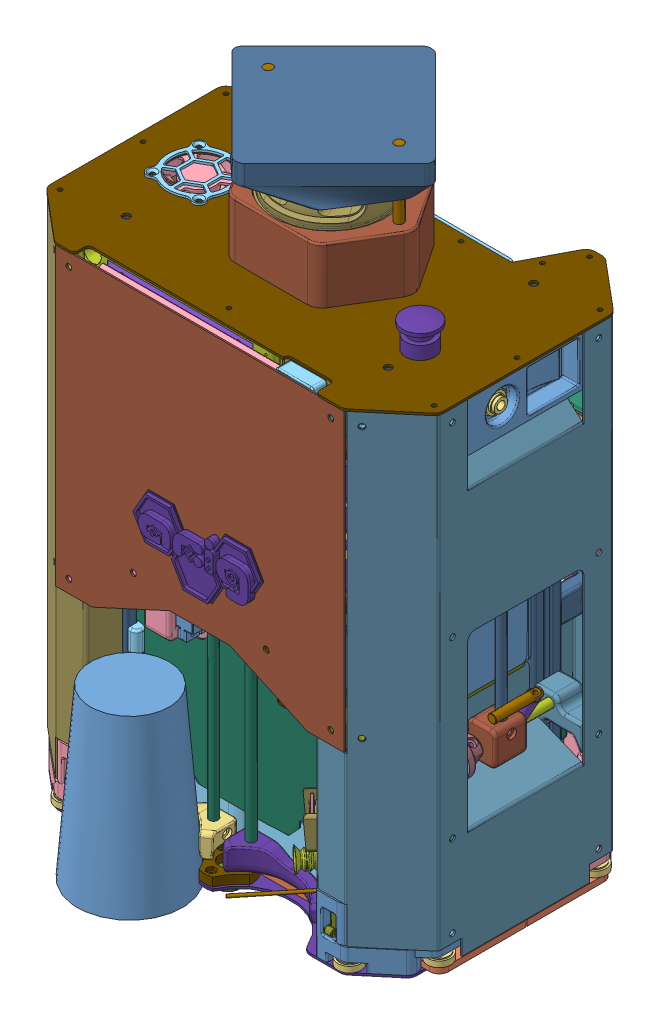
SolidWorks assembly _2021_RobotSecondaire_V1, configuration Default. Lengths in mm. (continued)
Components (placement in the parent): (continued)
- _Symétrie_Angle-4: _Symétrie_Angle [Défaut] at (-3.845 0 0) x (-1 0 0) z (0 0 -1) size (53.5 52 51.1)
  - _Symétrie_microswitchGaletAss-1: _Symétrie_microswitchGaletAss [Défaut] at (85.155 44 -75) x (0 -1 0) z (1 0 0) size (21.06 21.1 7)
    - _Symétrie_microswitchGalet02-1: _Symétrie_microswitchGalet02 [Défaut] at origin size (20 15 7)
    - _Symétrie_microswitchGalet01-1: _Symétrie_microswitchGalet01 [Défaut] at (1.7099 12.1145 0) x (0.996636 -0.081957 0) z (0 0 1) size (19 9 6)
  - _Symétrie_Angle_support-1: _Symétrie_Angle_support [Défaut] at (86.155 7 -50) size (53.5 52 49)
- PlaqueAvant-2: PlaqueAvant [Défaut] at (0 5.5 -40) x (-1 0 0) z (0 0 -1) size (250 17.2 51.5)
  - BillePorteuse2019-1: BillePorteuse2019 [Défaut] at (0 -6.2 30) size (16 10 16)
  - PlaqueAvant_Tole-1: PlaqueAvant_Tole [Défaut] at origin size (250 1.5 50)
  - PlaqueAvant_SupportBille-1: PlaqueAvant_SupportBille [Défaut] at (0 2.5 30) size (32 10 25.6)
  - RoulementAngle-1: RoulementAngle [Défaut] at (-96.8842 4.25 43.5) size (16 9.5 16)
  - RoulementAngle-2: RoulementAngle [Défaut] at (96.8842 4.25 43.5) size (16 9.5 16)
- _Symétrie_BrasLateral-2: _Symétrie_BrasLateral [Défaut] at (82 117.5 38.35) size (52.5 125.87 147.5)
  - _Symétrie_Access_HS-645_Rond-1: _Symétrie_Access_HS-645_Rond [Défaut] at (28 -10.2 -7.8) x (-0.986286 0.165048 0) z (-0.165048 -0.986286 0) size (24 5 24)
  - _Symétrie_Servo_HS-485-HB-1: _Symétrie_Servo_HS-485-HB [Default] at (28 -10.2 31.94) x (-1 0 0) z (0 0 1) size (19.81 54.15 42.74)
  - _Symétrie_Bras_AxePivot-1: _Symétrie_Bras_AxePivot [Default] at (28 -10.2 -16.3) x (0.492424 0.870356 0) z (0 0 1) size (6 6 80)
  - _Symétrie_Bras_Alu_TubeCarre_07.5-1: _Symétrie_Bras_Alu_TubeCarre_07.5 [Default] at (34.6477 1.5498 -55.3) x (0.870356 -0.492424 0) z (0.492424 0.870356 0) size (8 8 26)
  - _Symétrie_Bras_AxeButee-1: _Symétrie_Bras_AxeButee [Default] at (41.2954 13.2996 -59.3) x (0.492424 0.870356 0) z (0 0 -1) size (6 6 33)
  - _Symétrie_Bras_Rouleau-1: _Symétrie_Bras_Rouleau [Défaut] at (35.2953 -10.2 -38.75) x (0 0 -1) z (0 -1 0) size (24.5 22.96 102.46)
    - _Symétrie_Bras_Axe-1: _Symétrie_Bras_Axe [Default] at origin size (6 6 94)
    - _Symétrie_Bras_Pivot-1: _Symétrie_Bras_Pivot [Default] at (0 0 8) x (0 1 0) z (-1 0 0) size (22.5 23 22.5)
    - _Symétrie_Igus_Bague_d06-1: _Symétrie_Igus_Bague_d06 [Défaut] at (-12.25 -7.2953 0) size (10 12 12)
    - _Symétrie_Igus_Bague_d06-2: _Symétrie_Igus_Bague_d06 [Défaut] at (12.25 -7.2953 0) x (-1 0 0) z (0 0.759835 -0.650115) size (10 12 12)
  - _Symétrie_Bras_FixAxePivot-1: _Symétrie_Bras_FixAxePivot [Défaut] at (28 -10.2 -12.3) x (-0.870356 0.492424 0) z (-0.492424 -0.870356 0) size (24 14 24)
  - _Symétrie_Bras_SupportAxe-1: _Symétrie_Bras_SupportAxe [Défaut] at (18 -21.2 -88.35) x (0 0 -1) z (-1 0 0) size (18 26 35)
  - _Symétrie_Bras_SupportServo_Bottom-1: _Symétrie_Bras_SupportServo_Bottom [Défaut] at (8 -42.065 11.65) x (0 0 1) z (-1 0 0) size (18 22 35)
  - _Symétrie_Bras_SupportServo_Top-1: _Symétrie_Bras_SupportServo_Top [Défaut] at (8 19.815 11.65) x (-1 0 0) z (0 0 -1) size (39 18 44.5)
- LogoARIG2-1: LogoARIG2 [Défaut] at (-42.5 182 89.5) size (88.08 45.8 6.03)
- LogoARIG2-3: LogoARIG2 [Défaut] at (42.5 182 -89.5) x (-1 0 0) z (0 0 -1) size (88.08 45.8 6.03)
- Pneumatique2-2: Pneumatique2 [Défaut] at (-80 92 0) x (0 0 -1) z (1 0 0) size (118 63.5 92.8)
  - Pneumatique_Support2-1: Pneumatique_Support2 [Défaut] at (0 0 -10) size (118 15 27.1)
  - CroixPiquageRapideD06-1: CroixPiquageRapideD06 [Default] at (12.5 14.5 29.25) x (-1 0 0) z (0 -1 0) size (38 38 13)
  - CroixPiquageRapideD06-2: CroixPiquageRapideD06 [Default] at (-12.5 -6.5 29.25) x (1 0 0) z (0 1 0) size (38 38 13)
  - CapteurVide_CKD_PPE-V01A-H6-B-1: CapteurVide_CKD_PPE-V01A-H6-B [Défaut] at (12.5 14.5 52.75) x (0 -1 0) z (-1 0 0) size (37 43 15)
  - CapteurVide_CKD_PPE-V01A-H6-B-2: CapteurVide_CKD_PPE-V01A-H6-B [Défaut] at (-12.5 -6.5 52.75) x (0 1 0) z (1 0 0) size (37 43 15)
  - Electrovanne_CylindriqueD24_NC_12V-1: Electrovanne_CylindriqueD24_NC_12V [Default] at (12.5 -18.5 -2) x (0 0 1) z (-1 0 0) size (38.24 53 24.48)
  - Electrovanne_CylindriqueD24_NC_12V-2: Electrovanne_CylindriqueD24_NC_12V [Default] at (-12.5 26.5 -2) x (0 0 1) z (1 0 0) size (38.24 53 24.48)
  - Pneumatique_Fix-1: Pneumatique_Fix [Défaut] at (0 0 -2) x (-1 0 0) z (0 0 -1) size (75 8 14.55)
  - Pièce4^Pneumatique2-1: Pièce4^Pneumatique2 [Défaut] at (-9 -6.5 29.25) x (0 -1 0) z (1 0 0) size (24.78 14.3 44.64) (virtual)
  - Pièce5^Pneumatique2-1: Pièce5^Pneumatique2 [Défaut] at (16 14.5 29.25) x (0 -1 0) z (1 0 0) size (50.6 27.61 36.51) (virtual)
  - Pièce6^Pneumatique2-1: Pièce6^Pneumatique2 [Défaut] at (-16 -6.5 29.25) x (0 1 0) z (-1 0 0) size (29.52 27.83 36.35) (virtual)
  - Pièce7^Pneumatique2-1: Pièce7^Pneumatique2 [Défaut] at (9 14.5 29.25) x (0 1 0) z (-1 0 0) size (45.5 14.26 63.44) (virtual)
Mates (geometry in assembly coordinates):
- Coïncidente1: coincident: plane of assembly through (0 0 0) normal (0 1 0); plane of 2020_ADJ_Bouee-1 through (37.5 0 100) normal (0 1 0); plane of assembly
- Coïncidente2: coincident: plane of assembly through (0 0 0) normal (0 1 0); plane of 2020_ADJ_Bouee-2 through (-37.5 0 100) normal (0 1 0); plane of assembly
- Coïncidente3: coincident: plane of assembly through (0 0 0) normal (0 1 0); plane of 2020_ADJ_Bouee-3 through (37.5 0 -100) normal (0 1 0); plane of assembly
- Coïncidente4: coincident: plane of assembly through (0 0 0) normal (0 1 0); plane of 2020_ADJ_Bouee-4 through (-37.5 0 -100) normal (0 1 0); plane of assembly
- Coïncidente5: coincident: plane of assembly; plane of assembly; plane of 2020_ADJ_Bouee-1 through (37.5 0 100) normal (0 0 1); plane of 2020_ADJ_Bouee-2 through (-37.5 0 100) normal (0 0 1)
- Coïncidente6: coincident: plane of assembly; plane of assembly; plane of 2020_ADJ_Bouee-3 through (37.5 0 -100) normal (0 0 1); plane of 2020_ADJ_Bouee-4 through (-37.5 0 -100) normal (0 0 1)
- Coïncidente7: coincident: plane of assembly; plane of assembly; plane of 2020_ADJ_Bouee-1 through (37.5 0 100) normal (1 0 0); plane of 2020_ADJ_Bouee-3 through (37.5 0 -100) normal (1 0 0)
- Coïncidente8: coincident: plane of assembly; plane of assembly; plane of 2020_ADJ_Bouee-2 through (-37.5 0 100) normal (1 0 0); plane of 2020_ADJ_Bouee-4 through (-37.5 0 -100) normal (1 0 0)
- Symétrique1: symmetric: plane of assembly; plane of assembly; plane of 2020_ADJ_Bouee-1 through (37.5 0 100) normal (1 0 0); plane of 2020_ADJ_Bouee-2 through (-37.5 0 100) normal (1 0 0); plane of assembly
- Symétrique2: symmetric: plane of assembly; plane of assembly; plane of 2020_ADJ_Bouee-1 through (37.5 0 100) normal (0 0 1); plane of 2020_ADJ_Bouee-3 through (37.5 0 -100) normal (0 0 1); plane of assembly
- Distance1: distance = 100 mm: plane of assembly through (0 0 0) normal (0 0 1); plane of 2020_ADJ_Bouee-1 through (37.5 0 100) normal (0 0 1); plane of assembly
- Distance2: distance = 37.5 mm: plane of assembly through (0 0 0) normal (1 0 0); plane of 2020_ADJ_Bouee-1 through (37.5 0 100) normal (1 0 0); plane of assembly
- Coïncidente73: coincident: plane of VolumeRobot-1 through (0 0 0) normal (0 0 1); plane of assembly through (0 0 0) normal (0 0 1)
- Coïncidente74: coincident: plane of VolumeRobot-1 through (0 0 0) normal (0 1 0); plane of assembly through (0 0 0) normal (0 1 0)
- Coïncidente75: coincident: plane of VolumeRobot-1 through (0 0 0) normal (1 0 0); plane of assembly through (0 0 0) normal (1 0 0)
- Coïncidente77: coincident: plane of assembly; plane of assembly; plane of ProfiléX20_330-4 through (99.2 11 46.7) normal (0 -1 0); plane of BaseRoulante-1/BaseRoulante_Plaque-1 through (0 11 0) normal (0 1 0)
- Coïncidente78: coincident: plane of assembly; plane of assembly; plane of ProfiléX20_330-4 through (86.7 341 60) normal (0 0 1); plane of BaseRoulante-1/BaseRoulante_Plaque-1 through (0 11 60) normal (0 0 1)
- Coaxiale23: concentric: circle of assembly; circle of assembly; circle of ProfiléX20_330-4; circle of BaseRoulante-1/BaseRoulante_Plaque-1
- Coïncidente79: coincident: plane of assembly; plane of assembly; plane of ProfiléX20_330-3 through (-86.7 11 59.2) normal (0 -1 0); plane of BaseRoulante-1/BaseRoulante_Plaque-1 through (0 11 0) normal (0 1 0)
- Coaxiale24: concentric: circle of assembly; circle of assembly; circle of ProfiléX20_330-3; circle of BaseRoulante-1/BaseRoulante_Plaque-1
- Coïncidente80: coincident: plane of assembly; plane of assembly; plane of ProfiléX20_330-3 through (-93.3 341 60) normal (0 0 1); plane of BaseRoulante-1/BaseRoulante_Plaque-1 through (0 11 60) normal (0 0 1)
- Coïncidente81: coincident: plane of assembly; plane of assembly; plane of ProfiléX20_330-2 through (-86.7 341 -60) normal (0 0 -1); plane of BaseRoulante-1/BaseRoulante_Plaque-1 through (0 11 -60) normal (0 0 -1)
- Coïncidente82: coincident: plane of assembly; plane of assembly; plane of ProfiléX20_330-2 through (-86.7 11 -40.8) normal (0 -1 0); plane of BaseRoulante-1/BaseRoulante_Plaque-1 through (0 11 0) normal (0 1 0)
- Coaxiale25: concentric: circle of assembly; circle of assembly; circle of ProfiléX20_330-2; circle of BaseRoulante-1/BaseRoulante_Plaque-1
- Coaxiale26: concentric: circle of assembly; circle of assembly; circle of ProfiléX20_330-1; circle of BaseRoulante-1/BaseRoulante_Plaque-1
- Coïncidente83: coincident: plane of assembly; plane of assembly; plane of ProfiléX20_330-1 through (93.3 11 -40.8) normal (0 -1 0); plane of BaseRoulante-1/BaseRoulante_Plaque-1 through (0 11 0) normal (0 1 0)
- Coïncidente84: coincident: plane of assembly; plane of assembly; plane of ProfiléX20_330-1 through (82 341 -60) normal (0 0 -1); plane of BaseRoulante-1/BaseRoulante_Plaque-1 through (0 11 -60) normal (0 0 -1)
- Coïncidente208: coincident: plane of assembly; plane of assembly; plane of ProfiléX20_330-4 through (99.2 341 46.7) normal (0 1 0); plane of BlocSup-1/BlocSup_Plaque-1 through (0 341 0) normal (0 -1 0)
- Coaxiale56: concentric: circle of assembly; circle of assembly; circle of ProfiléX20_330-4; circle of BlocSup-1/BlocSup_Plaque-1
- Coaxiale57: concentric: circle of assembly; circle of assembly; circle of ProfiléX20_330-2; circle of BlocSup-1/BlocSup_Plaque-1
- Coïncidente213: coincident: plane of BlocSup-1/Lidar-1/Lidar_Base-1 through (0 342.5 0) normal (0 0 1); plane of assembly through (0 0 0) normal (0 0 1)
- Coïncidente214: coincident: plane of BlocSup-1/Lidar-1/Lidar_Base-1 through (0 342.5 0) normal (1 0 0); plane of assembly through (0 0 0) normal (1 0 0)
- Coïncidente330: coincident: plane of assembly through (0 0 0) normal (1 0 0); plane of PompeVide-AirpoD2028B-12vdc-1 through (0 51 59.6) normal (1 0 0); plane of assembly
- Coïncidente331: coincident: plane of assembly through (0 0 0) normal (1 0 0); plane of PompeVide-AirpoD2028B-12vdc-2 through (0 51 21) normal (-1 0 0); plane of assembly
- Distance81: distance = 1 mm: plane of assembly; plane of assembly; plane of BaseRoulante-1/BaseRoulante_Plaque-1 through (0 11 0) normal (0 1 0); plane of PompeVide-AirpoD2028B-12vdc-2 through (0 12 59.6) normal (0 -1 0)
- Distance80: distance = 1 mm: plane of assembly; plane of assembly; plane of BaseRoulante-1/BaseRoulante_Plaque-1 through (0 11 0) normal (0 1 0); plane of PompeVide-AirpoD2028B-12vdc-1 through (0 12 21) normal (0 -1 0)
- Coïncidente334: coincident: plane of ? through (-60 31 21) normal (0 0 1); plane of PompeVide-AirpoD2028B-12vdc-1 through (-62.4 51 21) normal (0 0 -1)
- Coïncidente335: coincident: plane of ? through (60 31 21) normal (0 0 1); plane of PompeVide-AirpoD2028B-12vdc-2 through (0 51 21) normal (0 0 -1)
- Coïncidente340: coincident: plane of assembly; plane of assembly; plane of ProfiléX20_330-2 through (-98 341 -60) normal (0 0 -1); plane of BlocVentouse-2/BlocVentouse_SupportVentouse-1 through (-92.35 56 -60) normal (0 0 1)
- Coïncidente341: coincident: plane of assembly; plane of assembly; plane of BlocVentouse-1/BlocVentouse_SupportCapteurCouleur-1 through (80.4705 83 73.1713) normal (0 1 0); plane of BlocVentouse-2/BlocVentouse_SupportCapteurCouleur-1 through (-80.4705 83 -73.1713) normal (0 1 0)
- Coïncidente342: coincident: plane of assembly; plane of assembly; plane of ProfiléX20_330-3 through (-82 341 60) normal (0 0 1); plane of _Symétrie_BlocVentouse-3/_Symétrie_BlocVentouse_SupportVentouse-1 through (-87.65 56 60) normal (0 0 -1)
- Distance78: distance = 0.5 mm: plane of assembly; plane of assembly; plane of ProfiléX20_330-3 through (-80 341 53.3) normal (1 0 0); plane of _Symétrie_BlocVentouse-3/_Symétrie_BlocVentouse_SupportVentouse-1 through (-79.5 56 60) normal (-1 0 0)
- Coïncidente344: coincident: plane of assembly; plane of assembly; plane of BlocVentouse-1/BlocVentouse_SupportCapteurCouleur-1 through (80.4705 83 73.1713) normal (0 1 0); plane of _Symétrie_BlocVentouse-3/_Symétrie_BlocVentouse_SupportCapteurCouleur-1 through (-80.4705 83 73.1713) normal (0 1 0)
- Distance79: distance = 0.5 mm: plane of assembly; plane of assembly; plane of ProfiléX20_330-1 through (80 341 -53.3) normal (-1 0 0); plane of _Symétrie_BlocVentouse-4/_Symétrie_BlocVentouse_SupportVentouse-1 through (79.5 56 -60) normal (1 0 0)
- Coïncidente347: coincident: plane of assembly; plane of assembly; plane of ProfiléX20_330-1 through (82 341 -60) normal (0 0 -1); plane of _Symétrie_BlocVentouse-4/_Symétrie_BlocVentouse_SupportVentouse-1 through (92.35 56 -60) normal (0 0 1)
- Coïncidente348: coincident: plane of assembly; plane of assembly; plane of BlocVentouse-1/BlocVentouse_SupportCapteurCouleur-1 through (80.4705 83 73.1713) normal (0 1 0); plane of _Symétrie_BlocVentouse-4/_Symétrie_BlocVentouse_SupportCapteurCouleur-1 through (80.4705 83 -73.1713) normal (0 1 0)
- Distance52: distance = 117.5 mm: plane of assembly through (0 0 0) normal (0 1 0); plane of BrasLateral-1 through (-82 117.5 38.35) normal (0 1 0); plane of assembly
- Coïncidente368: coincident: plane of assembly; plane of assembly; plane of ProfiléX20_330-2 through (-82 341 -40) normal (0 0 1); plane of Tole_Centre-5 through (0 153.5 -40) normal (0 0 -1)
- Coaxiale151: concentric: cylinder of assembly; cylinder of assembly; cylinder of Tole_Centre-5 through (-51.2 177.5 -38.499) axis (0 0 -1) radius 1.6; cylinder of PouseGobelet-3/PouseGobelet_SupportServo-1 through (-51.2 177.5 -40) axis (0 0 1) radius 1.25
- Coïncidente369: coincident: plane of assembly; plane of assembly; plane of Tole_Centre-5 through (0 153.5 -40) normal (0 0 -1); plane of PouseGobelet-3/PouseGobelet_SupportServo-1 through (-54.7 173.75 -40) normal (0 0 1)
- Coïncidente370: coincident: plane of assembly; plane of assembly; plane of Tole_Centre-5 through (0 153.5 -40) normal (0 0 -1); plane of _Symétrie_PouseGobelet-3/_Symétrie_PouseGobelet_SupportServo-1 through (54.7 173.75 -40) normal (0 0 1)
- Coaxiale152: concentric: cylinder of assembly; cylinder of assembly; cylinder of Tole_Centre-5 through (-40.2 177.5 -38.499) axis (0 0 -1) radius 1.6; cylinder of PouseGobelet-3/PouseGobelet_SupportServo-1 through (-40.2 177.5 -40) axis (0 0 1) radius 1.25
- Coaxiale153: concentric: cylinder of assembly; cylinder of assembly; cylinder of Tole_Centre-5 through (40.2 177.5 -38.499) axis (0 0 -1) radius 1.6; cylinder of _Symétrie_PouseGobelet-3/_Symétrie_PouseGobelet_SupportServo-1 through (40.2 177.5 -40) axis (0 0 1) radius 1.25
- Coaxiale154: concentric: cylinder of assembly; cylinder of assembly; cylinder of Tole_Centre-5 through (51.2 177.5 -38.499) axis (0 0 -1) radius 1.6; cylinder of _Symétrie_PouseGobelet-3/_Symétrie_PouseGobelet_SupportServo-1 through (51.2 177.5 -40) axis (0 0 1) radius 1.25
- Distance53: distance = 2 mm: plane of assembly; plane of assembly; plane of ProfiléX20_330-1 through (100 341 -46.7) normal (1 0 0); plane of Tole_Centre-5 through (98 126 -40) normal (1 0 0)
- Coïncidente381: coincident: plane of assembly; plane of assembly; plane of Tole_Centre-5 through (-98 181 -40) normal (0 1 0); plane of Batterie-2/Batterie_Logement_Top-2 through (0 181 0) normal (0 1 0)
- Coïncidente427: coincident: plane of assembly; plane of assembly; plane of ProfiléX20_330-2 through (-93.3 341 -40) normal (0 0 1); plane of Pneumatique-6/Pneumatique_Support-1 through (-65 77.5 -40) normal (0 0 -1)
- Coïncidente428: coincident: plane of assembly; plane of assembly; plane of BaseRoulante-1/BaseRoulante_ToleCarter-1 through (-61 67.5 0) normal (0 1 0); plane of Pneumatique-6/Pneumatique_Support-1 through (-90 67.5 0) normal (0 -1 0)
- Distance59: distance = 1 mm: plane of assembly; plane of assembly; plane of Pneumatique-6/Pneumatique_Support-1 through (-99 77.5 -40) normal (-1 0 0); plane of ProfiléX20_330-3 through (-100 341 46.7) normal (-1 0 0)
- Coïncidente429: coincident: plane of assembly; plane of assembly; plane of ProfiléX20_330-2 through (-93.3 341 -40) normal (0 0 1); plane of Pneumatique-6/Pneumatique_Top-1 through (-80 97.5 -40) normal (0 0 -1)
- Coïncidente430: coincident: plane of assembly; plane of assembly; plane of BaseRoulante-1/BaseRoulante_Plaque-1 through (0 7 0) normal (0 -1 0); plane of PlaqueAvant-1/PlaqueAvant_Tole-1 through (0 7 40) normal (0 1 0)
- Coaxiale163: concentric: cylinder of assembly; cylinder of assembly; cylinder of BaseRoulante-1/BaseRoulante_Plaque-1 through (115 6.999 45) axis (0 1 0) radius 1.25; cylinder of PlaqueAvant-1/PlaqueAvant_Tole-1 through (115 5.5 45) axis (0 1 0) radius 1
- Coïncidente441: coincident: plane of assembly; plane of assembly; plane of PlaqueAvant-1/PlaqueAvant_Tole-1 through (0 7 40) normal (0 1 0); plane of Angle-1/Angle_support-1 through (90 7 50) normal (0 -1 0)
- Coïncidente443: coincident: plane of assembly; plane of assembly; plane of PlaqueAvant-1/PlaqueAvant_Tole-1 through (0 7 90) normal (0 0 1); plane of Angle-1/Angle_support-1 through (90 47 90) normal (0 0 1)
- Distance60: distance = 1.5 mm: plane of assembly; plane of assembly; plane of Angle-1/Angle_support-1 through (96.9164 -27.2344 90) normal (0.642788 0 0.766044); plane of PlaqueAvant-1/PlaqueAvant_Tole-1 through (65.6279 7 118.2123) normal (0.642788 0 0.766044)
- Coïncidente446: coincident: plane of assembly; plane of assembly; plane of ProfiléX20_330-2 through (-98 341 -60) normal (0 0 -1); plane of Carter_FixAngle-1 through (-99 137.315 -60) normal (0 0 1)
- Distance61: distance = 1 mm: plane of assembly; plane of assembly; plane of Carter_FixAngle-1 through (-99 137.315 -60) normal (-1 0 0); plane of ProfiléX20_330-2 through (-100 341 -53.3) normal (-1 0 0)
- Distance62: distance = 45 mm: plane of assembly; plane of assembly; plane of BlocVentouse-2/BlocVentouse_SupportVentouse-1 through (-37.5 56 -100) normal (0 1 0); plane of BaseRoulante-1/BaseRoulante_Plaque-1 through (0 11 0) normal (0 1 0)
- Coïncidente450: coincident: plane of assembly; plane of assembly; plane of ProfiléX20_330-2 through (-86.7 341 -60) normal (0 0 -1); plane of Angle-2/Angle_support-1 through (-90 47 -60) normal (0 0 1)
- Coïncidente451: coincident: plane of assembly; plane of assembly; plane of PlaqueAvant-2/PlaqueAvant_Tole-1 through (0 7 -40) normal (0 1 0); plane of Angle-2/Angle_support-1 through (-90 7 -50) normal (0 -1 0)
- Coïncidente453: coincident: plane of assembly; plane of assembly; plane of ProfiléX20_330-1 through (93.3 341 -60) normal (0 0 -1); plane of _Symétrie_Angle-3/_Symétrie_Angle_support-1 through (90 47 -60) normal (0 0 1)
- Coïncidente454: coincident: plane of assembly; plane of assembly; plane of PlaqueAvant-2/PlaqueAvant_Tole-1 through (0 7 -40) normal (0 1 0); plane of _Symétrie_Angle-3/_Symétrie_Angle_support-1 through (90 7 -50) normal (0 -1 0)
- Distance64: distance = 1.5 mm: plane of assembly; plane of assembly; plane of PlaqueAvant-2/PlaqueAvant_Tole-1 through (65.6279 7 -118.2123) normal (0.642788 0 -0.766044); plane of _Symétrie_Angle-3/_Symétrie_Angle_support-1 through (96.9164 -27.2344 -90) normal (0.642788 0 -0.766044)
- Coïncidente456: coincident: plane of assembly; plane of assembly; plane of ProfiléX20_330-3 through (-93.3 341 60) normal (0 0 1); plane of _Symétrie_Angle-4/_Symétrie_Angle_support-1 through (-90 47 60) normal (0 0 -1)
- Coïncidente457: coincident: plane of assembly; plane of assembly; plane of PlaqueAvant-1/PlaqueAvant_Tole-1 through (0 7 40) normal (0 1 0); plane of _Symétrie_Angle-4/_Symétrie_Angle_support-1 through (-90 7 50) normal (0 -1 0)
- Distance65: distance = 1.5 mm: plane of assembly; plane of assembly; plane of _Symétrie_Angle-4/_Symétrie_Angle_support-1 through (-96.9164 -27.2344 90) normal (-0.642788 0 0.766044); plane of PlaqueAvant-1/PlaqueAvant_Tole-1 through (-65.6279 7 118.2123) normal (-0.642788 0 0.766044)
- Coïncidente459: coincident: plane of assembly; plane of assembly; plane of Carter_FixAngle-1 through (-90 155.315 -60) normal (0 1 0); plane of _Symétrie_Carter_FixAngle-4 through (90 155.315 -60) normal (0 1 0)
- Coïncidente460: coincident: plane of assembly; plane of assembly; plane of ProfiléX20_330-1 through (93.3 341 -60) normal (0 0 -1); plane of _Symétrie_Carter_FixAngle-4 through (87.65 137.315 -60) normal (0 0 1)
- Distance67: distance = 1 mm: plane of assembly; plane of assembly; plane of ProfiléX20_330-1 through (100 341 -58) normal (1 0 0); plane of _Symétrie_Carter_FixAngle-4 through (99 137.315 -60) normal (1 0 0)
- Coïncidente470: coincident: plane of assembly; plane of assembly; plane of ProfiléX20_330-3 through (-93.3 341 60) normal (0 0 1); plane of BrasLateral-1/Bras_SupportServo_Top-1 through (-90 155.315 60) normal (0 0 -1)
- Coïncidente471: coincident: plane of assembly; plane of assembly; plane of ProfiléX20_330-3 through (-100 341 58) normal (-1 0 0); plane of BrasLateral-1/Bras_SupportServo_Bottom-1 through (-100 93.435 41) normal (1 0 0)
- Coïncidente480: coincident: plane of assembly through (0 0 0) normal (1 0 0); plane of CarterAvant-1 through (0 137.5 88.5) normal (1 0 0); plane of assembly
- Coïncidente481: coincident: plane of assembly; plane of assembly; plane of CarterAvant-1 through (0 341 88.5) normal (0 1 0); plane of BlocSup-1/BlocSup_Plaque-1 through (0 341 0) normal (0 -1 0)
- Coïncidente482: coincident: plane of assembly; plane of assembly; plane of BaseRoulante-1/BaseRoulante_Plaque-1 through (0 11 0) normal (0 1 0); plane of CarterDroite-1 through (-133.1428 11 -59.5834) normal (0 -1 0)
- Coïncidente483: coincident: plane of assembly; plane of assembly; plane of BlocSup-1/BlocSup_CarterDroite-1 through (-133.5 341 -59.3005) normal (-1 0 0); plane of CarterDroite-1 through (-133.5 341 -59.75) normal (1 0 0)
- Coïncidente484: coincident: plane of assembly through (0 0 0) normal (0 0 1); plane of CarterDroite-1 through (-134.5 11 0) normal (0 0 1); plane of assembly
- Coïncidente489: coincident: plane of assembly; plane of assembly; plane of ProfiléX20_330-4 through (98 341 60) normal (0 0 1); plane of MatDrapeau-1/MatDrapeau_SupportServo_Droite-1 through (99 341 60) normal (0 0 -1)
- Distance73: distance = 1 mm: plane of assembly; plane of assembly; plane of ProfiléX20_330-4 through (100 341 53.3) normal (1 0 0); plane of MatDrapeau-1/MatDrapeau_SupportServo_Droite-1 through (99 341 60) normal (1 0 0)
- Coïncidente491: coincident: plane of assembly; plane of assembly; plane of BlocSup-1/BlocSup_Plaque-1 through (0 341 0) normal (0 -1 0); plane of MatDrapeau-1/MatDrapeau_SupportServo_Droite-1 through (90 341 50) normal (0 1 0)
- Coïncidente492: coincident: plane of assembly; plane of assembly; plane of MatDrapeau-1/MatDrapeau_SupportServo_Gauche-1 through (-99 341 88.5) normal (0 0 1); plane of CarterAvant-1 through (-99 341 88.5) normal (0 0 -1)
- Coïncidente493: coincident: plane of assembly; plane of assembly; plane of _Symétrie_Carter_FixAngle-4 through (90 155.315 -60) normal (0 1 0); plane of _Symétrie_BrasLateral-2/_Symétrie_Bras_SupportServo_Top-1 through (90 155.315 50) normal (0 1 0)
- Coïncidente494: coincident: plane of assembly through (0 0 0) normal (1 0 0); plane of CarterArriere-1 through (0 137.5 -88.5) normal (1 0 0); plane of assembly
- Coïncidente495: coincident: plane of assembly; plane of assembly; plane of BlocSup-1/_Symétrie_BlocSup_SupportCharniere-3 through (99 243 -88.5) normal (0 0 -1); plane of CarterArriere-1 through (-99 341 -88.5) normal (0 0 1)
- Coïncidente496: coincident: plane of assembly; plane of assembly; plane of CarterArriere-1 through (-99 243 -89.5) normal (0 1 0); plane of BlocSup-1/BlocSup_CarterEcran-1 through (99.3418 243 -90) normal (0 -1 0)
- Coïncidente498: coincident: plane of assembly; plane of assembly; plane of BaseRoulante-1/BaseRoulante_ToleCarter-2 through (61 67.5 0) normal (0 1 0); plane of Pneumatique-7/Pneumatique_Support-1 through (90 67.5 0) normal (0 -1 0)
- Coïncidente499: coincident: plane of assembly; plane of assembly; plane of ProfiléX20_330-1 through (98 341 -40) normal (0 0 1); plane of Pneumatique-7/Pneumatique_Top-1 through (99 97.5 -40) normal (0 0 -1)
- Distance74: distance = 1 mm: plane of assembly; plane of assembly; plane of Pneumatique-7/Pneumatique_Top-1 through (99 97.5 40) normal (1 0 0); plane of ProfiléX20_330-4 through (100 341 42) normal (1 0 0)
- Coïncidente501: coincident: plane of assembly; plane of assembly; plane of CarterAvant-1 through (-99 341 89.5) normal (0 0 1); plane of LogoARIG2-1 through (-42.5 182 89.5) normal (0 0 -1)
- Parallèle22: parallel: plane of assembly through (0 0 0) normal (0 1 0); plane of LogoARIG2-1 through (-42.5 182 89.5) normal (0 1 0); plane of assembly
- Coïncidente507: coincident: plane of assembly; plane of assembly; plane of Tole_Centre-5 through (-98 181 -40) normal (0 1 0); plane of Tole_Centre-6 through (-98 181 38.5) normal (0 1 0)
- Coïncidente508: coincident: plane of assembly through (0 0 0) normal (1 0 0); plane of Tole_Centre-6 through (0 153.5 40) normal (1 0 0); plane of assembly
- Distance75: distance = 170 mm: plane of assembly; plane of assembly; plane of Tole_Centre-5 through (-98 181 -40) normal (0 1 0); plane of BaseRoulante-1/BaseRoulante_Plaque-1 through (0 11 0) normal (0 1 0)
- Coïncidente510: coincident: plane of assembly; plane of assembly; plane of ProfiléX20_330-4 through (93.3 341 40) normal (0 0 -1); plane of Tole_Centre-6 through (0 153.5 40) normal (0 0 1)
- Coaxiale164: concentric: cylinder of assembly; cylinder of assembly; cylinder of PouseGobelet-1/PouseGobelet_SupportServo-1 through (51.2 177.5 40) axis (0 0 -1) radius 1.25; cylinder of Tole_Centre-6 through (51.2 177.5 40.001) axis (0 0 -1) radius 1.6
- Coaxiale165: concentric: cylinder of assembly; cylinder of assembly; cylinder of PouseGobelet-1/PouseGobelet_SupportServo-1 through (40.2 177.5 40) axis (0 0 -1) radius 1.25; cylinder of Tole_Centre-6 through (40.2 177.5 40.001) axis (0 0 -1) radius 1.6
- Coïncidente511: coincident: plane of assembly; plane of assembly; plane of PouseGobelet-1/PouseGobelet_SupportServo-1 through (54.7 173.75 40) normal (0 0 -1); plane of Tole_Centre-6 through (0 153.5 40) normal (0 0 1)
- Coaxiale166: concentric: cylinder of assembly; cylinder of assembly; cylinder of _Symétrie_PouseGobelet-4/_Symétrie_PouseGobelet_SupportServo-1 through (-40.2 177.5 40) axis (0 0 -1) radius 1.25; cylinder of Tole_Centre-6 through (-40.2 177.5 40.001) axis (0 0 -1) radius 1.6
- Coaxiale167: concentric: cylinder of assembly; cylinder of assembly; cylinder of _Symétrie_PouseGobelet-4/_Symétrie_PouseGobelet_SupportServo-1 through (-51.2 177.5 40) axis (0 0 -1) radius 1.25; cylinder of Tole_Centre-6 through (-51.2 177.5 40.001) axis (0 0 -1) radius 1.6
- Coïncidente512: coincident: plane of assembly; plane of assembly; plane of _Symétrie_PouseGobelet-4/_Symétrie_PouseGobelet_SupportServo-1 through (-54.7 173.75 40) normal (0 0 -1); plane of Tole_Centre-6 through (0 153.5 40) normal (0 0 1)
- Parallèle23: parallel: plane of assembly through (0 0 0) normal (0 1 0); plane of Batterie-2/batterieLIPO-1 through (-78.5499 135.881 20.8896) normal (0 -1 0); plane of assembly
- Coïncidente516: coincident: plane of assembly; plane of assembly; plane of BrasLateral-1/Bras_SupportServo_Top-1 through (-90 145.315 50) normal (0 1 0); plane of _Symétrie_BrasLateral-2/_Symétrie_Bras_SupportServo_Top-1 through (90 145.315 50) normal (0 1 0)
- Coïncidente517: coincident: plane of assembly; plane of assembly; plane of CarterDroite-1 through (-134.5 11 0) normal (0 0 1); plane of CarterGauche-1 through (134.5 11 0) normal (0 0 -1)
- Coïncidente518: coincident: plane of assembly; plane of assembly; plane of BlocSup-1/BlocSup_CarterGauche-1 through (133.5 341 59.3005) normal (1 0 0); plane of CarterGauche-1 through (133.5 341 59.75) normal (-1 0 0)
- Coïncidente519: coincident: plane of assembly; plane of assembly; plane of CarterDroite-1 through (-134.5 11 0) normal (0 1 0); plane of CarterGauche-1 through (134.5 11 0) normal (0 1 0)
- Coïncidente521: coincident: plane of assembly through (0 0 0) normal (1 0 0); plane of CarterPompes-1 through (0 39 -372.943) normal (1 0 0); plane of assembly
- Coïncidente522: coincident: plane of assembly through (0 0 0) normal (1 0 0); plane of CarterPompes-2 through (0 39 372.943) normal (-1 0 0); plane of assembly
- Coïncidente523: coincident: plane of assembly; plane of assembly; plane of CarterPompes-1 through (0 139 -372.943) normal (0 1 0); plane of CarterPompes-2 through (0 139 372.943) normal (0 1 0)
- Coïncidente524: coincident: plane of assembly; plane of assembly; plane of ProfiléX20_330-2 through (-80 341 -58) normal (1 0 0); plane of Angle-2/Angle_support-1 through (-80 47 -50) normal (1 0 0)
- Coïncidente526: coincident: plane of assembly; plane of assembly; plane of ProfiléX20_330-4 through (98 341 60) normal (0 0 1); plane of BlocVentouse-1/BlocVentouse_SupportVentouse-1 through (92.35 56 60) normal (0 0 -1)
- Distance76: distance = 0.5 mm: plane of assembly; plane of assembly; plane of ProfiléX20_330-4 through (80 341 58) normal (-1 0 0); plane of BlocVentouse-1/BlocVentouse_SupportVentouse-1 through (79.5 56 60) normal (1 0 0)
- Distance77: distance = 0.5 mm: plane of assembly; plane of assembly; plane of ProfiléX20_330-2 through (-80 341 -58) normal (1 0 0); plane of BlocVentouse-2/BlocVentouse_SupportVentouse-1 through (-79.5 56 -60) normal (-1 0 0)
- Coïncidente538: coincident: plane of assembly; plane of assembly; plane of ProfiléX20_330-4 through (80 341 46.7) normal (-1 0 0); plane of Pneumatique2-1/Pneumatique_Support2-1 through (80 100 -47.65) normal (1 0 0)
- Distance82: distance = 1 mm: plane of assembly; plane of assembly; plane of ProfiléX20_330-1 through (82 341 -60) normal (0 0 -1); plane of Pneumatique2-1/Pneumatique_Support2-1 through (74 100 -59) normal (0 0 -1)
- Distance83: distance = 2 mm: plane of assembly; plane of assembly; plane of Pneumatique2-1/Electrovanne_CylindriqueD24_NC_12V-2 through (79 69.5 -12.5) normal (0 -1 0); plane of BaseRoulante-1/BaseRoulante_ToleCarter-2 through (61 67.5 0) normal (0 1 0)
- Coïncidente539: coincident: plane of assembly; plane of assembly; plane of ProfiléX20_330-3 through (-80 341 53.3) normal (1 0 0); plane of Pneumatique2-2/Pneumatique_Support2-1 through (-80 100 59) normal (-1 0 0)
- Distance84: distance = 1 mm: plane of assembly; plane of assembly; plane of Pneumatique2-2/Pneumatique_Support2-1 through (-74 100 59) normal (0 0 1); plane of ProfiléX20_330-3 through (-82 341 60) normal (0 0 1)
- Coïncidente541: coincident: plane of assembly; plane of assembly; plane of Pneumatique2-1/Pneumatique_Support2-1 through (90 100 0) normal (0 1 0); plane of Pneumatique2-2/Pneumatique_Support2-1 through (-90 100 0) normal (0 1 0)
- Coïncidente542: coincident: plane of assembly; plane of assembly; plane of PompeVide-AirpoD2028B-12vdc-3 through (-62.4 51 -59.6) normal (0 0 -1); plane of PompeVide-AirpoD2028B-12vdc-4 through (0 51 -59.6) normal (0 0 -1)
- Coïncidente543: coincident: plane of assembly; plane of assembly; plane of BaseRoulante-1/BlocSuppMoteur2021-1 through (-13 46 -21) normal (0 0 -1); plane of PompeVide-AirpoD2028B-12vdc-3 through (0 51 -21) normal (0 0 1)
- Distance85: distance = 8 mm: point of assembly; plane of assembly; point of CarterPompes-2; plane of ProfiléX20_330-1 through (82 341 -60) normal (0 0 -1)
- Coïncidente545: coincident: plane of assembly; plane of assembly; plane of PompeVide-AirpoD2028B-12vdc-4 through (0 39 -59.6) normal (0 1 0); plane of CarterPompes-1 through (0 39 -372.943) normal (0 1 0)
- Distance86: distance = 8 mm: point of assembly; plane of assembly; point of CarterPompes-1; plane of ProfiléX20_330-3 through (-82 341 60) normal (0 0 1)
- Coaxiale168: concentric: cylinder of assembly; cylinder of assembly; cylinder of CarterAvant-1 through (30 206 88.5) axis (0 0 1) radius 2; cylinder of LogoARIG2-1 through (30 206 97.8941) axis (0 0 -1) radius 1.2
